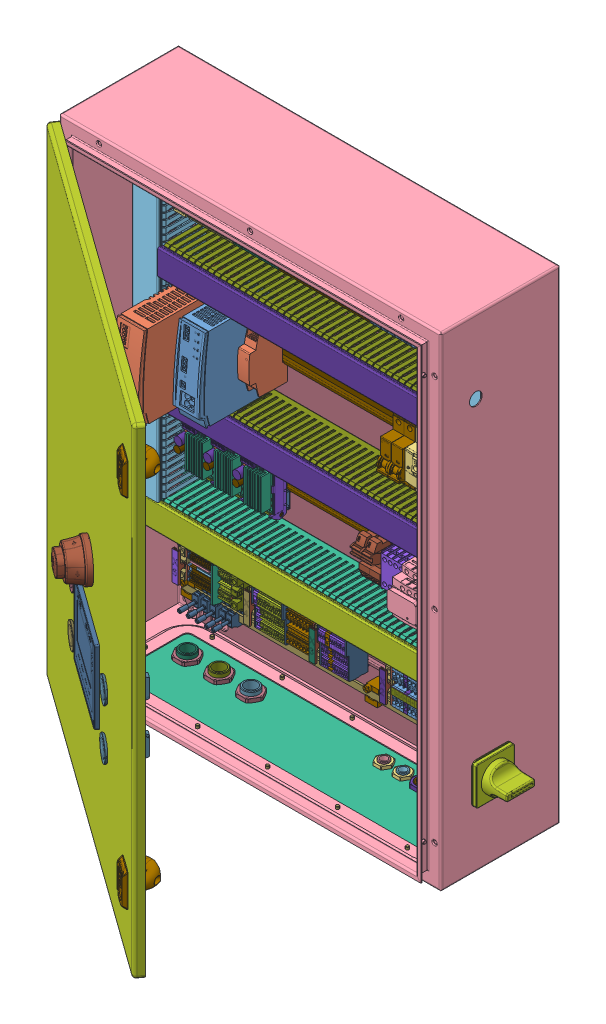
SolidWorks assembly Armoir életrique v46.step, configuration Valor predeterminado. Lengths in mm. (continued)
Components (placement in the parent): (continued)
- 37.5 X 75 Narrow Slot BASE WITH LID.step-1: 37.5 X 75 Narrow Slot BASE WITH LID.step [Valor predeterminado] at origin size (468 41.01 78.6)
  - Body1.step-1: Body1.step [Valor predeterminado] at (-551 554.8681 -521.8) x (0 -1 0) z (0 0 1) size (41 468 77)
  - Body2.step-1: Body2.step [Valor predeterminado] at (-551 554.8681 -521.8) x (0 -1 0) z (0 0 1) size (41.01 468 7.4)
- 37.5 X 75 Narrow Slot BASE WITH LID_1.step-1: 37.5 X 75 Narrow Slot BASE WITH LID_1.step [Valor predeterminado] at (0 -220 0) size (468 41.01 78.6)
  - Body1.step-1: Body1.step [Valor predeterminado] at (-551 593.8681 -521.8) x (0 -1 0) z (0 0 1) size (41 468 77)
  - Body2.step-1: Body2.step [Valor predeterminado] at (-551 593.8681 -521.8) x (0 -1 0) z (0 0 1) size (41.01 468 7.4)
- 1207653 466.step-1: 1207653 466.step [Valor predeterminado] at (0 375 125) size (466 35 7.5)
  - NS_35_7.5_PERF_955MM-select.step-1: NS_35_7.5_PERF_955MM-select.step [Valor predeterminado] at (125.3 207.4662 -151.4677) x (0 1 0) z (1 0 0) size (35 7.5 466)
- 1207653 466_1.step-1: 1207653 466_1.step [Valor predeterminado] at (0 145 125) size (466 35 7.5)
  - NS_35_7.5_PERF_955MM-select.step-1: NS_35_7.5_PERF_955MM-select.step [Valor predeterminado] at (126.3 85.9654 -151.4677) x (0 1 0) z (1 0 0) size (35 7.5 466)
- 2905743.step-1: 2905743.step [Valor predeterminado] at (0 550 200) size (41 130.04 121)
  - CBM_E4_24DC_0.5_10A_NO_R-select.step-1: CBM_E4_24DC_0.5_10A_NO_R-select.step [Valor predeterminado] at (132.998 -56.1004 -52.502) x (0 0 -1) z (0 -1 0) size (121 41 130.04)
- 2903149_TRIO_PS_2G_1AC_24DC_10-select.step-1: 2903149_TRIO_PS_2G_1AC_24DC_10-select.step [Valor predeterminado] at (50 625 200) x (0 1 0) z (1 0 0) size (130 167 42)
  - 2903149_TRIO_PS_2G_1AC_24DC_10-select_1.step-1: 2903149_TRIO_PS_2G_1AC_24DC_10-select_1.step [Valor predeterminado] at (-236.8504 -172.5 20.5) x (0 1 0) z (0 0 -1) size (167 130 42)
- 37.5 X 75 Narrow Slot BASE WITH LID_2.step-1: 37.5 X 75 Narrow Slot BASE WITH LID_2.step [Valor predeterminado] at (0 -500 0) size (468 41.01 78.6)
  - Body1.step-1: Body1.step [Valor predeterminado] at (-550 694.8677 -521.8) x (0 -1 0) z (0 0 1) size (41 468 77)
  - Body2.step-1: Body2.step [Valor predeterminado] at (-550 694.8677 -521.8) x (0 -1 0) z (0 0 1) size (41.01 468 7.4)
- 1207653 466_2.step-1: 1207653 466_2.step [Valor predeterminado] at (0 -145 125) size (466 35 7.5)
  - NS_35_7.5_PERF_955MM-select.step-1: NS_35_7.5_PERF_955MM-select.step [Valor predeterminado] at (125.3 544.9658 -151.4677) x (0 1 0) z (1 0 0) size (35 7.5 466)
- 2903334_RIF_1_RPT_LDP_24DC_2x21-select_1.step-1: 2903334_RIF_1_RPT_LDP_24DC_2x21-select_1.step [Valor predeterminado] at (240 390 50) x (0 1 0) z (1 0 0) size (104.84 89.77 16.3)
  - 2903334_RIF_1_RPT_LDP_24DC_2x21-select_2.step-1: 2903334_RIF_1_RPT_LDP_24DC_2x21-select_2.step [Valor predeterminado] at (-71.3019 -22.3322 159.95) x (-0.992546 -0.121869 0) z (0 0 -1) size (95.96 78.66 16.3)
- GV2ME16.step-1: GV2ME16.step [Valor predeterminado] at origin size (89 89 77.76)
  - GV2ME10-3D-SIMPLIFIED.step-1: GV2ME10-3D-SIMPLIFIED.step [Valor predeterminado] at (463.25 407.4996 47.5) size (44.5 89 77.76)
  - GV2ME10-3D-SIMPLIFIED.step-2: GV2ME10-3D-SIMPLIFIED.step [Valor predeterminado] at (507.75 407.4996 47.5) size (44.5 89 77.76)
- LC1D12BD.step-1: LC1D12BD.step [Valor predeterminado] at (700 300 0) size (89.6 77 94.65)
  - LC1D09-18C-DC.step-1: LC1D09-18C-DC.step [Valor predeterminado] at (-258.6 -55.7008 22) size (44.8 77 94.65)
  - LC1D09-18C-DC.step-2: LC1D09-18C-DC.step [Valor predeterminado] at (-213.8 -55.7008 22) size (44.8 77 94.65)
- 37.5 X 75 Narrow Slot BASE WITH LID_3.step-1: 37.5 X 75 Narrow Slot BASE WITH LID_3.step [Valor predeterminado] at origin size (41.01 529 78.6)
  - Body1_1.step-1: Body1_1.step [Valor predeterminado] at (211.6315 -337.5 -521.8) size (41.01 529 78.6)
- 37.5 X 75 Narrow Slot BASE WITH LID_4.step-1: 37.5 X 75 Narrow Slot BASE WITH LID_4.step [Valor predeterminado] at (350 0 0) size (41.01 529 78.6)
  - Body1_1.step-1: Body1_1.step [Valor predeterminado] at (370.6319 -337.5 -521.8) size (41.01 529 78.6)
- 37.5 X 75 Narrow Slot BASE WITH LID_5.step-1: 37.5 X 75 Narrow Slot BASE WITH LID_5.step [Valor predeterminado] at origin size (550 41.01 78.6)
  - Body1_2.step-1: Body1_2.step [Valor predeterminado] at (-510.0004 25.8681 -521.8) x (0 -1 0) z (0 0 1) size (41 550 77)
  - Body2_2.step-1: Body2_2.step [Valor predeterminado] at (-510.0004 25.8681 -521.8) x (0 -1 0) z (0 0 1) size (41.01 550 7.4)
- Rail bornier complet.step-1: Rail bornier complet.step [Valor predeterminado] at (531.5 121.5 20) x (-1 0 0) z (0 0 1) size (500.55 113.8 62.99)
  - Bornier X3.step-1: Bornier X3.step [Valor predeterminado] at (226.5 -28.5 -20) size (55.9 81.82 53.31)
    - pxc_3244449_03_PTIO-1-5-S-3-PE_3D.step-1: pxc_3244449_03_PTIO-1-5-S-3-PE_3D.step [Valor predeterminado] at origin size (3.5 81.82 53.31)
      - PTIO_1.5_S_3_PE-select.step-1: PTIO_1.5_S_3_PE-select.step [Valor predeterminado] at (9.4 -10.4554 38.8743) x (0 0.992546 -0.121869) z (1 0 0) size (77 44.26 3.5)
    - pxc_3244560_03_PTIO-IN-2-5-3-PE-OG_3D.step-1: pxc_3244560_03_PTIO-IN-2-5-3-PE-OG_3D.step [Valor predeterminado] at (12 0 0) size (7 74.4 40)
      - PTIO_IN_2.5_3_PE_OG-Select.step-1: PTIO_IN_2.5_3_PE_OG-Select.step [Valor predeterminado] at (-50.17 -12.4414 42.0332) x (0 1 0) z (1 0 0) size (74.4 40 7)
    - pxc_3244449_03_PTIO-1-5-S-3-PE_3D_1.step-1: pxc_3244449_03_PTIO-1-5-S-3-PE_3D_1.step [Valor predeterminado] at (-25 0 0) size (3.5 81.82 53.31)
      - PTIO_1.5_S_3_PE-select.step-1: PTIO_1.5_S_3_PE-select.step [Valor predeterminado] at (30.9 -10.4554 38.8743) x (0 0.992546 -0.121869) z (1 0 0) size (77 44.26 3.5)
    - pxc_3244449_03_PTIO-1-5-S-3-PE_3D_2.step-1: pxc_3244449_03_PTIO-1-5-S-3-PE_3D_2.step [Valor predeterminado] at (-45 0 0) size (3.5 81.82 53.31)
      - PTIO_1.5_S_3_PE-select.step-1: PTIO_1.5_S_3_PE-select.step [Valor predeterminado] at (64.9 -10.4554 38.8743) x (0 0.992546 -0.121869) z (1 0 0) size (77 44.26 3.5)
    - pxc_3244449_03_PTIO-1-5-S-3-PE_3D_3.step-1: pxc_3244449_03_PTIO-1-5-S-3-PE_3D_3.step [Valor predeterminado] at (-37 0 0) size (3.5 81.82 53.31)
      - PTIO_1.5_S_3_PE-select.step-1: PTIO_1.5_S_3_PE-select.step [Valor predeterminado] at (60.4 -10.4554 38.8743) x (0 0.992546 -0.121869) z (1 0 0) size (77 44.26 3.5)
    - pxc_3244449_03_PTIO-1-5-S-3-PE_3D_4.step-1: pxc_3244449_03_PTIO-1-5-S-3-PE_3D_4.step [Valor predeterminado] at (-60 0 0) size (3.5 81.82 53.31)
      - PTIO_1.5_S_3_PE-select.step-1: PTIO_1.5_S_3_PE-select.step [Valor predeterminado] at (62.4 -10.4554 38.8743) x (0 0.992546 -0.121869) z (1 0 0) size (77 44.26 3.5)
    - pxc_3244449_03_PTIO-1-5-S-3-PE_3D_5.step-1: pxc_3244449_03_PTIO-1-5-S-3-PE_3D_5.step [Valor predeterminado] at (-76 0 0) size (3.5 81.82 53.31)
      - PTIO_1.5_S_3_PE-select.step-1: PTIO_1.5_S_3_PE-select.step [Valor predeterminado] at (74.9 -10.4554 38.8743) x (0 0.992546 -0.121869) z (1 0 0) size (77 44.26 3.5)
    - pxc_3244449_03_PTIO-1-5-S-3-PE_3D_6.step-1: pxc_3244449_03_PTIO-1-5-S-3-PE_3D_6.step [Valor predeterminado] at (-93 0 0) size (3.5 81.82 53.31)
      - PTIO_1.5_S_3_PE-select.step-1: PTIO_1.5_S_3_PE-select.step [Valor predeterminado] at (88.4 -10.4554 38.8743) x (0 0.992546 -0.121869) z (1 0 0) size (77 44.26 3.5)
    - pxc_3244449_03_PTIO-1-5-S-3-PE_3D_7.step-1: pxc_3244449_03_PTIO-1-5-S-3-PE_3D_7.step [Valor predeterminado] at (-107 0 0) size (3.5 81.82 53.31)
      - PTIO_1.5_S_3_PE-select.step-1: PTIO_1.5_S_3_PE-select.step [Valor predeterminado] at (98.9 -10.4554 38.8743) x (0 0.992546 -0.121869) z (1 0 0) size (77 44.26 3.5)
    - pxc_3244449_03_PTIO-1-5-S-3-PE_3D_8.step-1: pxc_3244449_03_PTIO-1-5-S-3-PE_3D_8.step [Valor predeterminado] at (-121 0 0) size (3.5 81.82 53.31)
      - PTIO_1.5_S_3_PE-select.step-1: PTIO_1.5_S_3_PE-select.step [Valor predeterminado] at (109.4 -10.4554 38.8743) x (0 0.992546 -0.121869) z (1 0 0) size (77 44.26 3.5)
    - pxc_3244575_01_D-PTIO-1-5-S-3_3D.step-1: pxc_3244575_01_D-PTIO-1-5-S-3_3D.step [Valor predeterminado] at (5 -8 5) size (2.2 74.4 33.8)
      - D_PTIO_1.5_S_3-select.step-1: D_PTIO_1.5_S_3-select.step [Valor predeterminado] at (-28.27 26.0888 49.1305) x (0 1 0) z (1 0 0) size (74.4 33.8 2.2)
    - pxc_3244575_01_D-PTIO-1-5-S-3_3D_1.step-1: pxc_3244575_01_D-PTIO-1-5-S-3_3D_1.step [Valor predeterminado] at (-60 -8 5) size (2.2 74.4 33.8)
      - D_PTIO_1.5_S_3-select.step-1: D_PTIO_1.5_S_3-select.step [Valor predeterminado] at (-7.47 26.0888 49.1305) x (0 1 0) z (1 0 0) size (74.4 33.8 2.2)
    - pxc_1202577_02_E-UK-NS-35_3D.step-1: pxc_1202577_02_E-UK-NS-35_3D.step [Valor predeterminado] at (8 0 0) size (9.5 54 43.4)
      - pxc_1004348_03_KLM-A_3D.step-1: pxc_1004348_03_KLM-A_3D.step [Valor predeterminado] at (0 0 7) size (9.5 46 36.8)
        - KLM_A-select.step-1: KLM_A-select.step [Valor predeterminado] at (21.1 -2.3378 32.5) x (0 1 0) z (1 0 0) size (46 36.8 9.5)
      - E_UK_NS_35_select.step-1: E_UK_NS_35_select.step [Valor predeterminado] at (21.1 448.4984 -308.7806) x (0 1 0) z (1 0 0) size (54 34.6 9.5)
    - pxc_3244449_03_PTIO-1-5-S-3-PE_3D_9.step-1: pxc_3244449_03_PTIO-1-5-S-3-PE_3D_9.step [Valor predeterminado] at (-26 0 0) size (3.5 81.82 53.31)
      - PTIO_1.5_S_3_PE-select.step-1: PTIO_1.5_S_3_PE-select.step [Valor predeterminado] at (52.9 -10.4554 38.8743) x (0 0.992546 -0.121869) z (1 0 0) size (77 44.26 3.5)
    - pxc_3213125_03_FBS-10-3-5-BU_3D.step-1: pxc_3213125_03_FBS-10-3-5-BU_3D.step [Valor predeterminado] at (0 0 60) size (26.75 3 18.23)
      - FBS_10_3.5_BU-select.step-1: FBS_10_3.5_BU-select.step [Valor predeterminado] at (38.285 40.9822 6.575) x (0 -1 0) z (-1 0 0) size (3 18.22 26.75)
    - pxc_3213109_03_FBS-4-3-5-BU_3D.step-1: pxc_3213109_03_FBS-4-3-5-BU_3D.step [Valor predeterminado] at (0 0 40) size (12.75 3 18.23)
      - FBS_4_3.5_BU-select.step-1: FBS_4_3.5_BU-select.step [Valor predeterminado] at (-33.485 32.7678 26.575) x (0 1 0) z (1 0 0) size (3 18.22 12.75)
    - Etiquette X3.step-1: Etiquette X3.step [Valor predeterminado] at (38.6 65 64.5) x (-1 0 0) z (0 0 1) size (9.5 46 0.1)
  - Bornier Alim.step-1: Bornier Alim.step [Valor predeterminado] at (81.5 -28.5 -20) size (54.15 55.92 43.5)
    - pxc_1202577_02_E-UK-NS-35_3D_1.step-1: pxc_1202577_02_E-UK-NS-35_3D_1.step [Valor predeterminado] at (0 0 -44) size (9.5 54 43.4)
      - pxc_1004348_03_KLM-A_3D_1.step-1: pxc_1004348_03_KLM-A_3D_1.step [Valor predeterminado] at (0 0 7) size (9.5 46 36.8)
        - KLM_A-select.step-1: KLM_A-select.step [Valor predeterminado] at (-36.85 -2.3378 76.5) x (0 1 0) z (1 0 0) size (46 36.8 9.5)
      - E_UK_NS_35_select.step-1: E_UK_NS_35_select.step [Valor predeterminado] at (-36.85 448.4984 -264.7806) x (0 1 0) z (1 0 0) size (54 34.6 9.5)
    - pxc_1202577_02_E-UK-NS-35_3D_2.step-1: pxc_1202577_02_E-UK-NS-35_3D_2.step [Valor predeterminado] at (0 0 52) size (9.5 54 34.6)
      - E_UK_NS_35_select_1.step-1: E_UK_NS_35_select_1.step [Valor predeterminado] at (-81.5 448.4984 -360.7806) x (0 1 0) z (1 0 0) size (54 34.6 9.5)
    - pxc_3211766_13_PT-4-PE_3D.step-1: pxc_3211766_13_PT-4-PE_3D.step [Valor predeterminado] at origin size (6.15 55.9 35.25)
      - PT_4_PE-select.step-1: PT_4_PE-select.step [Valor predeterminado] at (-64.65 61.3 36.75) x (0 1 0) z (1 0 0) size (55.9 35.25 6.15)
    - pxc_3211760_14_PT-4-BU_3D.step-1: pxc_3211760_14_PT-4-BU_3D.step [Valor predeterminado] at (-12 0 0) size (6.15 55.9 35.25)
      - PT_4_BU-Select.step-1: PT_4_BU-Select.step [Valor predeterminado] at (-46.5 61.3 36.75) x (0 1 0) z (1 0 0) size (55.9 35.25 6.15)
    - pxc_3211757_14_PT-4_3D.step-1: pxc_3211757_14_PT-4_3D.step [Valor predeterminado] at (-30 0 0) size (6.15 55.9 35.25)
      - PT_4-Select.step-1: PT_4-Select.step [Valor predeterminado] at (-10.05 61.3 36.75) x (0 1 0) z (1 0 0) size (55.9 35.25 6.15)
    - pxc_3211757_14_PT-4_3D_1.step-1: pxc_3211757_14_PT-4_3D_1.step [Valor predeterminado] at (-43 0 0) size (6.15 55.9 35.25)
      - PT_4-Select.step-1: PT_4-Select.step [Valor predeterminado] at (-3.2 61.3 36.75) x (0 1 0) z (1 0 0) size (55.9 35.25 6.15)
    - pxc_3211757_14_PT-4_3D_2.step-1: pxc_3211757_14_PT-4_3D_2.step [Valor predeterminado] at (-54 0 0) size (6.15 55.9 35.25)
      - PT_4-Select.step-1: PT_4-Select.step [Valor predeterminado] at (1.65 61.3 36.75) x (0 1 0) z (1 0 0) size (55.9 35.25 6.15)
    - pxc_3030420_04_D-ST-4_3D.step-1: pxc_3030420_04_D-ST-4_3D.step [Valor predeterminado] at (-40 0 0) size (2.2 55.9 29.05)
      - D-ST4-Body.step-1: D-ST4-Body.step [Valor predeterminado] at (-32 2.4502 65.8799) x (0 1 0) z (1 0 0) size (55.9 29.05 2.2)
      - D-ST4_Bridge_element1.step-1: D-ST4_Bridge_element1.step [Valor predeterminado] at (-32 2.4502 65.8799) x (0 1 0) z (1 0 0) size (9.39 5.98 1.8)
    - pxc_3030420_04_D-ST-4_3D_1.step-1: pxc_3030420_04_D-ST-4_3D_1.step [Valor predeterminado] at (-40 0 0) size (2.2 55.9 29.05)
      - D-ST4-Body.step-1: D-ST4-Body.step [Valor predeterminado] at (0.95 2.4502 65.8799) x (0 1 0) z (1 0 0) size (55.9 29.05 2.2)
      - D-ST4_Bridge_element1.step-1: D-ST4_Bridge_element1.step [Valor predeterminado] at (0.95 2.4502 65.8799) x (0 1 0) z (1 0 0) size (9.39 5.98 1.8)
    - Reperage X1.step-1: Reperage X1.step [Valor predeterminado] at (-61 45 40) x (0 -1 0) z (-1 0 0) size (10.5 4.25 30.75)
      - pxc_1051414_01_ZB-6-LGS-L1-N-PE_3D.step-1: pxc_1051414_01_ZB-6-LGS-L1-N-PE_3D.step [Valor predeterminado] at origin size (10.5 4.2 6.15)
        - 1051003_ZB_6_UNBEDRUCKT-select.step-1: 1051003_ZB_6_UNBEDRUCKT-select.step [Valor predeterminado] at (1061.9663 -328.6937 -21.95) size (10.5 4.2 6.15)
      - pxc_1051414_01_ZB-6-LGS-L1-N-PE_3D_1.step-1: pxc_1051414_01_ZB-6-LGS-L1-N-PE_3D_1.step [Valor predeterminado] at (8 0 0) size (10.5 4.2 6.15)
        - 1051003_ZB_6_UNBEDRUCKT-select.step-1: 1051003_ZB_6_UNBEDRUCKT-select.step [Valor predeterminado] at (1053.9663 -328.6937 -15.8) size (10.5 4.2 6.15)
      - pxc_1051414_01_ZB-6-LGS-L1-N-PE_3D_2.step-1: pxc_1051414_01_ZB-6-LGS-L1-N-PE_3D_2.step [Valor predeterminado] at (16 0 0) size (10.5 4.2 6.15)
        - 1051003_ZB_6_UNBEDRUCKT-select.step-1: 1051003_ZB_6_UNBEDRUCKT-select.step [Valor predeterminado] at (1045.9663 -328.6937 -9.65) size (10.5 4.2 6.15)
      - pxc_1051414_01_ZB-6-LGS-L1-N-PE_3D_3.step-1: pxc_1051414_01_ZB-6-LGS-L1-N-PE_3D_3.step [Valor predeterminado] at (24 0 0) size (10.5 4.2 6.15)
        - 1051003_ZB_6_UNBEDRUCKT-select.step-1: 1051003_ZB_6_UNBEDRUCKT-select.step [Valor predeterminado] at (1037.9663 -328.6937 -3.5) size (10.5 4.2 6.15)
      - pxc_1051414_01_ZB-6-LGS-L1-N-PE_3D_4.step-1: pxc_1051414_01_ZB-6-LGS-L1-N-PE_3D_4.step [Valor predeterminado] at (33 0 0) size (10.5 4.2 6.15)
        - 1051003_ZB_6_UNBEDRUCKT-select.step-1: 1051003_ZB_6_UNBEDRUCKT-select.step [Valor predeterminado] at (1028.9663 -328.6937 2.65) size (10.5 4.2 6.15)
      - Etiquette X1 1.step-1: Etiquette X1 1.step [Valor predeterminado] at (-7.5185 17.85 -21.95) x (0 0 1) z (0 1 0) size (30.75 10.5 0.05)
    - Etiquette X1.step-1: Etiquette X1.step [Valor predeterminado] at (-27.35 65 64.5) x (-1 0 0) z (0 0 1) size (9.5 46 0.1)
  - Bornier X4.step-1: Bornier X4.step [Valor predeterminado] at (266.5 -28.5 -20) size (102.8 81.82 53.31)
    - pxc_1202577_02_E-UK-NS-35_3D_3.step-1: pxc_1202577_02_E-UK-NS-35_3D_3.step [Valor predeterminado] at (90 0 0) size (9.5 54 43.4)
      - pxc_1004348_03_KLM-A_3D_2.step-1: pxc_1004348_03_KLM-A_3D_2.step [Valor predeterminado] at (0 0 7) size (9.5 46 36.8)
        - KLM_A-select.step-1: KLM_A-select.step [Valor predeterminado] at (1.9 -2.3378 32.5) x (0 1 0) z (1 0 0) size (46 36.8 9.5)
      - E_UK_NS_35_select.step-1: E_UK_NS_35_select.step [Valor predeterminado] at (1.9 448.4984 -308.7806) x (0 1 0) z (1 0 0) size (54 34.6 9.5)
    - pxc_3244436_03_PTIO-1-5-S-3-LED-24-GN_3D.step-1: pxc_3244436_03_PTIO-1-5-S-3-LED-24-GN_3D.step [Valor predeterminado] at (60 0 55) size (3.5 81.82 53.31)
      - PTIO_1.5_S_3_LED_24_GN-select.step-1: PTIO_1.5_S_3_LED_24_GN-select.step [Valor predeterminado] at (22.7 -10.4554 -16.1257) x (0 0.992546 -0.121869) z (1 0 0) size (77 44.26 3.5)
    - pxc_3244436_03_PTIO-1-5-S-3-LED-24-GN_3D_1.step-1: pxc_3244436_03_PTIO-1-5-S-3-LED-24-GN_3D_1.step [Valor predeterminado] at (55 0 55) size (3.5 81.82 53.31)
      - PTIO_1.5_S_3_LED_24_GN-select.step-1: PTIO_1.5_S_3_LED_24_GN-select.step [Valor predeterminado] at (24.2 -10.4554 -16.1257) x (0 0.992546 -0.121869) z (1 0 0) size (77 44.26 3.5)
    - pxc_3244436_03_PTIO-1-5-S-3-LED-24-GN_3D_2.step-1: pxc_3244436_03_PTIO-1-5-S-3-LED-24-GN_3D_2.step [Valor predeterminado] at (50 0 55) size (3.5 81.82 53.31)
      - PTIO_1.5_S_3_LED_24_GN-select.step-1: PTIO_1.5_S_3_LED_24_GN-select.step [Valor predeterminado] at (25.7 -10.4554 -16.1257) x (0 0.992546 -0.121869) z (1 0 0) size (77 44.26 3.5)
    - pxc_3244436_03_PTIO-1-5-S-3-LED-24-GN_3D_3.step-1: pxc_3244436_03_PTIO-1-5-S-3-LED-24-GN_3D_3.step [Valor predeterminado] at (45 0 55) size (3.5 81.82 53.31)
      - PTIO_1.5_S_3_LED_24_GN-select.step-1: PTIO_1.5_S_3_LED_24_GN-select.step [Valor predeterminado] at (27.2 -10.4554 -16.1257) x (0 0.992546 -0.121869) z (1 0 0) size (77 44.26 3.5)
    - pxc_3244559_05_PTIO-IN-2-5-3-OG_3D.step-1: pxc_3244559_05_PTIO-IN-2-5-3-OG_3D.step [Valor predeterminado] at (85 0 55) size (7 74.4 40)
      - PTIO_IN_2.5_3_OG-select.step-1: PTIO_IN_2.5_3_OG-select.step [Valor predeterminado] at (-49.87 -12.4414 -12.9668) x (0 1 0) z (1 0 0) size (74.4 40 7)
    - pxc_3244436_03_PTIO-1-5-S-3-LED-24-GN_3D_4.step-1: pxc_3244436_03_PTIO-1-5-S-3-LED-24-GN_3D_4.step [Valor predeterminado] at (45 0 55) size (3.5 81.82 53.31)
      - PTIO_1.5_S_3_LED_24_GN-select.step-1: PTIO_1.5_S_3_LED_24_GN-select.step [Valor predeterminado] at (23.7 -10.4554 -16.1257) x (0 0.992546 -0.121869) z (1 0 0) size (77 44.26 3.5)
    - pxc_3244436_03_PTIO-1-5-S-3-LED-24-GN_3D_5.step-1: pxc_3244436_03_PTIO-1-5-S-3-LED-24-GN_3D_5.step [Valor predeterminado] at (35 0 55) size (3.5 81.82 53.31)
      - PTIO_1.5_S_3_LED_24_GN-select.step-1: PTIO_1.5_S_3_LED_24_GN-select.step [Valor predeterminado] at (30.2 -10.4554 -16.1257) x (0 0.992546 -0.121869) z (1 0 0) size (77 44.26 3.5)
    - pxc_3244436_03_PTIO-1-5-S-3-LED-24-GN_3D_6.step-1: pxc_3244436_03_PTIO-1-5-S-3-LED-24-GN_3D_6.step [Valor predeterminado] at (25 0 55) size (3.5 81.82 53.31)
      - PTIO_1.5_S_3_LED_24_GN-select.step-1: PTIO_1.5_S_3_LED_24_GN-select.step [Valor predeterminado] at (36.7 -10.4554 -16.1257) x (0 0.992546 -0.121869) z (1 0 0) size (77 44.26 3.5)
    - pxc_3244436_03_PTIO-1-5-S-3-LED-24-GN_3D_7.step-1: pxc_3244436_03_PTIO-1-5-S-3-LED-24-GN_3D_7.step [Valor predeterminado] at (20 0 55) size (3.5 81.82 53.31)
      - PTIO_1.5_S_3_LED_24_GN-select.step-1: PTIO_1.5_S_3_LED_24_GN-select.step [Valor predeterminado] at (38.2 -10.4554 -16.1257) x (0 0.992546 -0.121869) z (1 0 0) size (77 44.26 3.5)
    - pxc_3244436_03_PTIO-1-5-S-3-LED-24-GN_3D_8.step-1: pxc_3244436_03_PTIO-1-5-S-3-LED-24-GN_3D_8.step [Valor predeterminado] at (15 0 55) size (3.5 81.82 53.31)
      - PTIO_1.5_S_3_LED_24_GN-select.step-1: PTIO_1.5_S_3_LED_24_GN-select.step [Valor predeterminado] at (39.7 -10.4554 -16.1257) x (0 0.992546 -0.121869) z (1 0 0) size (77 44.26 3.5)
    - pxc_3244436_03_PTIO-1-5-S-3-LED-24-GN_3D_9.step-1: pxc_3244436_03_PTIO-1-5-S-3-LED-24-GN_3D_9.step [Valor predeterminado] at (10 0 55) size (3.5 81.82 53.31)
      - PTIO_1.5_S_3_LED_24_GN-select.step-1: PTIO_1.5_S_3_LED_24_GN-select.step [Valor predeterminado] at (41.2 -10.4554 -16.1257) x (0 0.992546 -0.121869) z (1 0 0) size (77 44.26 3.5)
    - pxc_3244436_03_PTIO-1-5-S-3-LED-24-GN_3D_10.step-1: pxc_3244436_03_PTIO-1-5-S-3-LED-24-GN_3D_10.step [Valor predeterminado] at (35 0 55) size (3.5 81.82 53.31)
      - PTIO_1.5_S_3_LED_24_GN-select.step-1: PTIO_1.5_S_3_LED_24_GN-select.step [Valor predeterminado] at (12.7 -10.4554 -16.1257) x (0 0.992546 -0.121869) z (1 0 0) size (77 44.26 3.5)
    - pxc_3244575_01_D-PTIO-1-5-S-3_3D_2.step-1: pxc_3244575_01_D-PTIO-1-5-S-3_3D_2.step [Valor predeterminado] at origin size (2.2 74.4 33.8)
      - D_PTIO_1.5_S_3-select.step-1: D_PTIO_1.5_S_3-select.step [Valor predeterminado] at (39.53 18.0888 54.1305) x (0 1 0) z (1 0 0) size (74.4 33.8 2.2)
    - pxc_3244575_01_D-PTIO-1-5-S-3_3D_3.step-1: pxc_3244575_01_D-PTIO-1-5-S-3_3D_3.step [Valor predeterminado] at (25 0 0) size (2.2 74.4 33.8)
      - D_PTIO_1.5_S_3-select.step-1: D_PTIO_1.5_S_3-select.step [Valor predeterminado] at (-33.17 18.0888 54.1305) x (0 1 0) z (1 0 0) size (74.4 33.8 2.2)
    - pxc_3212329_18_PT-2-5-OG_3D.step-1: pxc_3212329_18_PT-2-5-OG_3D.step [Valor predeterminado] at (75 0 0) size (5.15 55.36 46.64)
      - PT_2.5_OG-select.step-1: PT_2.5_OG-select.step [Valor predeterminado] at (-33 7.1011 27.6678) x (0 0.992546 -0.121869) z (1 0 0) size (50.77 40.76 5.15)
    - pxc_3212329_18_PT-2-5-OG_3D_1.step-1: pxc_3212329_18_PT-2-5-OG_3D_1.step [Valor predeterminado] at (60 0 0) size (5.15 55.36 46.64)
      - PT_2.5_OG-select.step-1: PT_2.5_OG-select.step [Valor predeterminado] at (-23.15 7.1011 27.6678) x (0 0.992546 -0.121869) z (1 0 0) size (50.77 40.76 5.15)
    - pxc_3212329_18_PT-2-5-OG_3D_2.step-1: pxc_3212329_18_PT-2-5-OG_3D_2.step [Valor predeterminado] at (47 0 0) size (5.15 55.36 46.64)
      - PT_2.5_OG-select.step-1: PT_2.5_OG-select.step [Valor predeterminado] at (-15.3 7.1011 27.6678) x (0 0.992546 -0.121869) z (1 0 0) size (50.77 40.76 5.15)
    - pxc_3212329_18_PT-2-5-OG_3D_3.step-1: pxc_3212329_18_PT-2-5-OG_3D_3.step [Valor predeterminado] at (36 0 0) size (5.15 55.36 46.64)
      - PT_2.5_OG-select.step-1: PT_2.5_OG-select.step [Valor predeterminado] at (-9.45 7.1011 27.6678) x (0 0.992546 -0.121869) z (1 0 0) size (50.77 40.76 5.15)
    - pxc_3212329_18_PT-2-5-OG_3D_4.step-1: pxc_3212329_18_PT-2-5-OG_3D_4.step [Valor predeterminado] at (26 0 0) size (5.15 55.36 46.64)
      - PT_2.5_OG-select.step-1: PT_2.5_OG-select.step [Valor predeterminado] at (-4.6 7.1011 27.6678) x (0 0.992546 -0.121869) z (1 0 0) size (50.77 40.76 5.15)
    - pxc_3212329_18_PT-2-5-OG_3D_5.step-1: pxc_3212329_18_PT-2-5-OG_3D_5.step [Valor predeterminado] at (14 0 0) size (5.15 55.36 46.64)
      - PT_2.5_OG-select.step-1: PT_2.5_OG-select.step [Valor predeterminado] at (2.25 7.1011 27.6678) x (0 0.992546 -0.121869) z (1 0 0) size (50.77 40.76 5.15)
    - pxc_3212329_18_PT-2-5-OG_3D_6.step-1: pxc_3212329_18_PT-2-5-OG_3D_6.step [Valor predeterminado] at (14 0 0) size (5.15 55.36 46.64)
      - PT_2.5_OG-select.step-1: PT_2.5_OG-select.step [Valor predeterminado] at (-2.9 7.1011 27.6678) x (0 0.992546 -0.121869) z (1 0 0) size (50.77 40.76 5.15)
    - pxc_3212329_18_PT-2-5-OG_3D_7.step-1: pxc_3212329_18_PT-2-5-OG_3D_7.step [Valor predeterminado] at (4 0 0) size (5.15 55.36 46.64)
      - PT_2.5_OG-select.step-1: PT_2.5_OG-select.step [Valor predeterminado] at (1.95 7.1011 27.6678) x (0 0.992546 -0.121869) z (1 0 0) size (50.77 40.76 5.15)
    - pxc_3030417_05_D-ST-2-5_3D.step-1: pxc_3030417_05_D-ST-2-5_3D.step [Valor predeterminado] at (-5 0 0) size (2.2 48.6 29.05)
      - D-ST_2.5-Bridge_element1.step-1: D-ST_2.5-Bridge_element1.step [Valor predeterminado] at (3.6 6.3703 65.9) x (0 1 0) z (1 0 0) size (9.44 6 1.8)
      - D-ST_2.5-Body.step-1: D-ST_2.5-Body.step [Valor predeterminado] at (3.6 6.3703 65.9) x (0 1 0) z (1 0 0) size (48.6 29.05 2.2)
    - Etiquette X4.step-1: Etiquette X4.step [Valor predeterminado] at (101.4 65 64.5) x (-1 0 0) z (0 0 1) size (9.5 46 0.1)
  - 1207653.step-1: 1207653.step [Valor predeterminado] at (81.5 -28.5 -20) size (480 35 7.5)
    - NS_35_7.5_PERF_955MM-select_1.step-1: NS_35_7.5_PERF_955MM-select_1.step [Valor predeterminado] at (-20.2 -9.0338 -26.4677) x (0 1 0) z (1 0 0) size (35 7.5 480)
  - Bornier X2 moteur.step-1: Bornier X2 moteur.step [Valor predeterminado] at (112.5 -28.5 -20) size (100 55.92 43.5)
    - pxc_1202577_02_E-UK-NS-35_3D_4.step-1: pxc_1202577_02_E-UK-NS-35_3D_4.step [Valor predeterminado] at (0 0 -109) size (9.5 54 43.4)
      - pxc_1004348_03_KLM-A_3D_3.step-1: pxc_1004348_03_KLM-A_3D_3.step [Valor predeterminado] at (0 0 7) size (9.5 46 36.8)
        - KLM_A-select.step-1: KLM_A-select.step [Valor predeterminado] at (32.15 -2.3378 141.5) x (0 1 0) z (1 0 0) size (46 36.8 9.5)
      - E_UK_NS_35_select.step-1: E_UK_NS_35_select.step [Valor predeterminado] at (32.15 448.4984 -199.7806) x (0 1 0) z (1 0 0) size (54 34.6 9.5)
    - pxc_3211757_14_PT-4_3D_3.step-1: pxc_3211757_14_PT-4_3D_3.step [Valor predeterminado] at origin size (6.15 55.9 35.25)
      - PT_4-Select.step-1: PT_4-Select.step [Valor predeterminado] at (-26.4 61.3 36.75) x (0 1 0) z (1 0 0) size (55.9 35.25 6.15)
    - pxc_3211760_14_PT-4-BU_3D_1.step-1: pxc_3211760_14_PT-4-BU_3D_1.step [Valor predeterminado] at (-15 0 0) size (6.15 55.9 35.25)
      - PT_4_BU-Select.step-1: PT_4_BU-Select.step [Valor predeterminado] at (-5.25 61.3 36.75) x (0 1 0) z (1 0 0) size (55.9 35.25 6.15)
    - pxc_3211766_13_PT-4-PE_3D_1.step-1: pxc_3211766_13_PT-4-PE_3D_1.step [Valor predeterminado] at (19 0 0) size (6.15 55.9 35.25)
      - PT_4_PE-select.step-1: PT_4_PE-select.step [Valor predeterminado] at (-33.1 61.3 36.75) x (0 1 0) z (1 0 0) size (55.9 35.25 6.15)
    - pxc_3211766_13_PT-4-PE_3D_2.step-1: pxc_3211766_13_PT-4-PE_3D_2.step [Valor predeterminado] at (-51 0 70) size (6.15 55.9 35.25)
      - PT_4_PE-select.step-1: PT_4_PE-select.step [Valor predeterminado] at (0 61.3 -33.25) x (0 1 0) z (1 0 0) size (55.9 35.25 6.15)
    - pxc_3211766_13_PT-4-PE_3D_3.step-1: pxc_3211766_13_PT-4-PE_3D_3.step [Valor predeterminado] at (19 0 75) size (6.15 55.9 35.25)
      - PT_4_PE-select.step-1: PT_4_PE-select.step [Valor predeterminado] at (-8.5 61.3 -38.25) x (0 1 0) z (1 0 0) size (55.9 35.25 6.15)
    - pxc_3211757_14_PT-4_3D_4.step-1: pxc_3211757_14_PT-4_3D_4.step [Valor predeterminado] at origin size (6.15 55.9 35.25)
      - PT_4-Select.step-1: PT_4-Select.step [Valor predeterminado] at (-1.8 61.3 36.75) x (0 1 0) z (1 0 0) size (55.9 35.25 6.15)
    - pxc_3211757_14_PT-4_3D_5.step-1: pxc_3211757_14_PT-4_3D_5.step [Valor predeterminado] at origin size (6.15 55.9 35.25)
      - PT_4-Select.step-1: PT_4-Select.step [Valor predeterminado] at (16.65 61.3 36.75) x (0 1 0) z (1 0 0) size (55.9 35.25 6.15)
    - pxc_3211757_14_PT-4_3D_6.step-1: pxc_3211757_14_PT-4_3D_6.step [Valor predeterminado] at origin size (6.15 55.9 35.25)
      - PT_4-Select.step-1: PT_4-Select.step [Valor predeterminado] at (28.95 61.3 36.75) x (0 1 0) z (1 0 0) size (55.9 35.25 6.15)
    - pxc_3211757_14_PT-4_3D_7.step-1: pxc_3211757_14_PT-4_3D_7.step [Valor predeterminado] at origin size (6.15 55.9 35.25)
      - PT_4-Select.step-1: PT_4-Select.step [Valor predeterminado] at (4.35 61.3 36.75) x (0 1 0) z (1 0 0) size (55.9 35.25 6.15)
    - pxc_3211757_14_PT-4_3D_8.step-1: pxc_3211757_14_PT-4_3D_8.step [Valor predeterminado] at origin size (6.15 55.9 35.25)
      - PT_4-Select.step-1: PT_4-Select.step [Valor predeterminado] at (22.8 61.3 36.75) x (0 1 0) z (1 0 0) size (55.9 35.25 6.15)
    - pxc_3211757_14_PT-4_3D_9.step-1: pxc_3211757_14_PT-4_3D_9.step [Valor predeterminado] at origin size (6.15 55.9 35.25)
      - PT_4-Select.step-1: PT_4-Select.step [Valor predeterminado] at (-7.95 61.3 36.75) x (0 1 0) z (1 0 0) size (55.9 35.25 6.15)
    - pxc_3030420_04_D-ST-4_3D_2.step-1: pxc_3030420_04_D-ST-4_3D_2.step [Valor predeterminado] at (0 0 60) size (2.2 55.9 29.05)
      - D-ST4-Body.step-1: D-ST4-Body.step [Valor predeterminado] at (29.95 2.4502 5.8799) x (0 1 0) z (1 0 0) size (55.9 29.05 2.2)
      - D-ST4_Bridge_element1.step-1: D-ST4_Bridge_element1.step [Valor predeterminado] at (29.95 2.4502 5.8799) x (0 1 0) z (1 0 0) size (9.39 5.98 1.8)
    - pxc_3030420_04_D-ST-4_3D_3.step-1: pxc_3030420_04_D-ST-4_3D_3.step [Valor predeterminado] at (-110 0 60) size (2.2 55.9 29.05)
      - D-ST4-Body.step-1: D-ST4-Body.step [Valor predeterminado] at (51.65 2.4502 5.8799) x (0 1 0) z (1 0 0) size (55.9 29.05 2.2)
      - D-ST4_Bridge_element1.step-1: D-ST4_Bridge_element1.step [Valor predeterminado] at (51.65 2.4502 5.8799) x (0 1 0) z (1 0 0) size (9.39 5.98 1.8)
    - pxc_3211757_14_PT-4_3D_10.step-1: pxc_3211757_14_PT-4_3D_10.step [Valor predeterminado] at (85 0 0) size (6.15 55.9 35.25)
      - PT_4-Select.step-1: PT_4-Select.step [Valor predeterminado] at (-129.85 61.3 36.75) x (0 1 0) z (1 0 0) size (55.9 35.25 6.15)
    - pxc_3211760_14_PT-4-BU_3D_2.step-1: pxc_3211760_14_PT-4-BU_3D_2.step [Valor predeterminado] at (70 0 0) size (6.15 55.9 35.25)
      - PT_4_BU-Select.step-1: PT_4_BU-Select.step [Valor predeterminado] at (-108.7 61.3 36.75) x (0 1 0) z (1 0 0) size (55.9 35.25 6.15)
    - pxc_3211766_13_PT-4-PE_3D_4.step-1: pxc_3211766_13_PT-4-PE_3D_4.step [Valor predeterminado] at (104 0 0) size (6.15 55.9 35.25)
      - PT_4_PE-select.step-1: PT_4_PE-select.step [Valor predeterminado] at (-136.55 61.3 36.75) x (0 1 0) z (1 0 0) size (55.9 35.25 6.15)
    - pxc_3036958_04_FBS-4-6-BU_3D.step-1: pxc_3036958_04_FBS-4-6-BU_3D.step [Valor predeterminado] at (0 0 65) size (23.1 3 22.98)
      - FBS_4_6_BU-select.step-1: FBS_4_6_BU-select.step [Valor predeterminado] at (17.36 43.9967 1.225) x (0 -1 0) z (-1 0 0) size (3 22.97 23.1)
    - pxc_3030255_06_FBS-4-6_3D.step-1: pxc_3030255_06_FBS-4-6_3D.step [Valor predeterminado] at origin size (23.1 3 22.98)
      - FBS_4-6_select.step-1: FBS_4-6_select.step [Valor predeterminado] at (11.21 38.9822 66.225) x (0 -1 0) z (-1 0 0) size (3 22.98 23.1)
    - Reperage X2.step-1: Reperage X2.step [Valor predeterminado] at (0 0 72) size (86.1 10.5 4.25)
      - pxc_1051414_01_ZB-6-LGS-L1-N-PE_3D_5.step-1: pxc_1051414_01_ZB-6-LGS-L1-N-PE_3D_5.step [Valor predeterminado] at (29.95 52.5185 -18.35) x (-1 0 0) z (0 0 1) size (6.15 10.5 4.2)
        - 1051003_ZB_6_UNBEDRUCKT-select.step-1: 1051003_ZB_6_UNBEDRUCKT-select.step [Valor predeterminado] at (0 1069.4848 -342.3437) x (0 1 0) z (1 0 0) size (10.5 4.2 6.15)
      - pxc_1051414_01_ZB-6-LGS-L1-N-PE_3D_6.step-1: pxc_1051414_01_ZB-6-LGS-L1-N-PE_3D_6.step [Valor predeterminado] at (23.8 52.5185 -18.35) x (-1 0 0) z (0 0 1) size (6.15 10.5 4.2)
        - 1051003_ZB_6_UNBEDRUCKT-select.step-1: 1051003_ZB_6_UNBEDRUCKT-select.step [Valor predeterminado] at (0 1069.4848 -342.3437) x (0 1 0) z (1 0 0) size (10.5 4.2 6.15)
      - pxc_1051414_01_ZB-6-LGS-L1-N-PE_3D_7.step-1: pxc_1051414_01_ZB-6-LGS-L1-N-PE_3D_7.step [Valor predeterminado] at (17.65 52.5185 -18.35) x (-1 0 0) z (0 0 1) size (6.15 10.5 4.2)
        - 1051003_ZB_6_UNBEDRUCKT-select.step-1: 1051003_ZB_6_UNBEDRUCKT-select.step [Valor predeterminado] at (0 1069.4848 -342.3437) x (0 1 0) z (1 0 0) size (10.5 4.2 6.15)
      - pxc_1051414_01_ZB-6-LGS-L1-N-PE_3D_8.step-1: pxc_1051414_01_ZB-6-LGS-L1-N-PE_3D_8.step [Valor predeterminado] at (11.5 52.5185 -18.35) x (-1 0 0) z (0 0 1) size (6.15 10.5 4.2)
        - 1051003_ZB_6_UNBEDRUCKT-select.step-1: 1051003_ZB_6_UNBEDRUCKT-select.step [Valor predeterminado] at (0 1069.4848 -342.3437) x (0 1 0) z (1 0 0) size (10.5 4.2 6.15)
      - pxc_1051414_01_ZB-6-LGS-L1-N-PE_3D_9.step-1: pxc_1051414_01_ZB-6-LGS-L1-N-PE_3D_9.step [Valor predeterminado] at (5.35 52.5185 -18.35) x (-1 0 0) z (0 0 1) size (6.15 10.5 4.2)
        - 1051003_ZB_6_UNBEDRUCKT-select.step-1: 1051003_ZB_6_UNBEDRUCKT-select.step [Valor predeterminado] at (0 1069.4848 -342.3437) x (0 1 0) z (1 0 0) size (10.5 4.2 6.15)
      - pxc_1051414_01_ZB-6-LGS-L1-N-PE_3D_10.step-1: pxc_1051414_01_ZB-6-LGS-L1-N-PE_3D_10.step [Valor predeterminado] at (-0.8 52.5185 -18.35) x (-1 0 0) z (0 0 1) size (6.15 10.5 4.2)
        - 1051003_ZB_6_UNBEDRUCKT-select.step-1: 1051003_ZB_6_UNBEDRUCKT-select.step [Valor predeterminado] at (0 1069.4848 -342.3437) x (0 1 0) z (1 0 0) size (10.5 4.2 6.15)
      - pxc_1051414_01_ZB-6-LGS-L1-N-PE_3D_11.step-1: pxc_1051414_01_ZB-6-LGS-L1-N-PE_3D_11.step [Valor predeterminado] at (-6.95 52.5185 -18.35) x (-1 0 0) z (0 0 1) size (6.15 10.5 4.2)
        - 1051003_ZB_6_UNBEDRUCKT-select.step-1: 1051003_ZB_6_UNBEDRUCKT-select.step [Valor predeterminado] at (0 1069.4848 -342.3437) x (0 1 0) z (1 0 0) size (10.5 4.2 6.15)
      - pxc_1051414_01_ZB-6-LGS-L1-N-PE_3D_12.step-1: pxc_1051414_01_ZB-6-LGS-L1-N-PE_3D_12.step [Valor predeterminado] at (-13.1 52.5185 -18.35) x (-1 0 0) z (0 0 1) size (6.15 10.5 4.2)
        - 1051003_ZB_6_UNBEDRUCKT-select.step-1: 1051003_ZB_6_UNBEDRUCKT-select.step [Valor predeterminado] at (0 1069.4848 -342.3437) x (0 1 0) z (1 0 0) size (10.5 4.2 6.15)
      - pxc_1051414_01_ZB-6-LGS-L1-N-PE_3D_13.step-1: pxc_1051414_01_ZB-6-LGS-L1-N-PE_3D_13.step [Valor predeterminado] at (-19.25 52.5185 -18.35) x (-1 0 0) z (0 0 1) size (6.15 10.5 4.2)
        - 1051003_ZB_6_UNBEDRUCKT-select.step-1: 1051003_ZB_6_UNBEDRUCKT-select.step [Valor predeterminado] at (0 1069.4848 -342.3437) x (0 1 0) z (1 0 0) size (10.5 4.2 6.15)
      - pxc_1051414_01_ZB-6-LGS-L1-N-PE_3D_14.step-1: pxc_1051414_01_ZB-6-LGS-L1-N-PE_3D_14.step [Valor predeterminado] at (-25.4 52.5185 -18.35) x (-1 0 0) z (0 0 1) size (6.15 10.5 4.2)
        - 1051003_ZB_6_UNBEDRUCKT-select.step-1: 1051003_ZB_6_UNBEDRUCKT-select.step [Valor predeterminado] at (0 1069.4848 -342.3437) x (0 1 0) z (1 0 0) size (10.5 4.2 6.15)
      - pxc_1051414_01_ZB-6-LGS-L1-N-PE_3D_15.step-1: pxc_1051414_01_ZB-6-LGS-L1-N-PE_3D_15.step [Valor predeterminado] at (-31.55 52.5185 -18.35) x (-1 0 0) z (0 0 1) size (6.15 10.5 4.2)
        - 1051003_ZB_6_UNBEDRUCKT-select.step-1: 1051003_ZB_6_UNBEDRUCKT-select.step [Valor predeterminado] at (0 1069.4848 -342.3437) x (0 1 0) z (1 0 0) size (10.5 4.2 6.15)
      - pxc_1051414_01_ZB-6-LGS-L1-N-PE_3D_16.step-1: pxc_1051414_01_ZB-6-LGS-L1-N-PE_3D_16.step [Valor predeterminado] at (-37.7 52.5185 -18.35) x (-1 0 0) z (0 0 1) size (6.15 10.5 4.2)
        - 1051003_ZB_6_UNBEDRUCKT-select.step-1: 1051003_ZB_6_UNBEDRUCKT-select.step [Valor predeterminado] at (0 1069.4848 -342.3437) x (0 1 0) z (1 0 0) size (10.5 4.2 6.15)
      - pxc_1051414_01_ZB-6-LGS-L1-N-PE_3D_17.step-1: pxc_1051414_01_ZB-6-LGS-L1-N-PE_3D_17.step [Valor predeterminado] at (-43.85 52.5185 -18.35) x (-1 0 0) z (0 0 1) size (6.15 10.5 4.2)
        - 1051003_ZB_6_UNBEDRUCKT-select.step-1: 1051003_ZB_6_UNBEDRUCKT-select.step [Valor predeterminado] at (0 1069.4848 -342.3437) x (0 1 0) z (1 0 0) size (10.5 4.2 6.15)
      - pxc_1051414_01_ZB-6-LGS-L1-N-PE_3D_18.step-1: pxc_1051414_01_ZB-6-LGS-L1-N-PE_3D_18.step [Valor predeterminado] at (-50 52.5185 -18.35) x (-1 0 0) z (0 0 1) size (6.15 10.5 4.2)
        - 1051003_ZB_6_UNBEDRUCKT-select.step-1: 1051003_ZB_6_UNBEDRUCKT-select.step [Valor predeterminado] at (0 1069.4848 -342.3437) x (0 1 0) z (1 0 0) size (10.5 4.2 6.15)
      - Etiquette X2 1.step-1: Etiquette X2 1.step [Valor predeterminado] at (29.95 52.5185 -14.15) x (-1 0 0) z (0 0 1) size (86.1 10.5 0.05)
    - Etiquette X2.step-1: Etiquette X2.step [Valor predeterminado] at (41.65 65 64.5) x (-1 0 0) z (0 0 1) size (9.5 46 0.1)
  - Bornier X5.step-1: Bornier X5.step [Valor predeterminado] at (501.5 -28.5 120) size (92.1 59.9 48.62)
    - pxc_3208100_09_PT-1-5-S_3D.step-1: pxc_3208100_09_PT-1-5-S_3D.step [Valor predeterminado] at (-39 14 0) size (3.5 50.65 41.05)
      - PT_1.5_S-select.step-1: PT_1.5_S-select.step [Valor predeterminado] at (-8.2 -2.6891 -110.6257) x (0 0.992546 -0.121869) z (1 0 0) size (46.66 35.63 3.5)
    - pxc_3208100_09_PT-1-5-S_3D_1.step-1: pxc_3208100_09_PT-1-5-S_3D_1.step [Valor predeterminado] at (-39 14 0) size (3.5 50.65 41.05)
      - PT_1.5_S-select.step-1: PT_1.5_S-select.step [Valor predeterminado] at (-1.2 -2.6891 -110.6257) x (0 0.992546 -0.121869) z (1 0 0) size (46.66 35.63 3.5)
    - pxc_3208100_09_PT-1-5-S_3D_2.step-1: pxc_3208100_09_PT-1-5-S_3D_2.step [Valor predeterminado] at (-39 14 0) size (3.5 50.65 41.05)
      - PT_1.5_S-select.step-1: PT_1.5_S-select.step [Valor predeterminado] at (-4.7 -2.6891 -110.6257) x (0 0.992546 -0.121869) z (1 0 0) size (46.66 35.63 3.5)
    - pxc_3208100_09_PT-1-5-S_3D_3.step-1: pxc_3208100_09_PT-1-5-S_3D_3.step [Valor predeterminado] at (-39 14 0) size (3.5 50.65 41.05)
      - PT_1.5_S-select.step-1: PT_1.5_S-select.step [Valor predeterminado] at (2.3 -2.6891 -110.6257) x (0 0.992546 -0.121869) z (1 0 0) size (46.66 35.63 3.5)
    - pxc_3208100_09_PT-1-5-S_3D_4.step-1: pxc_3208100_09_PT-1-5-S_3D_4.step [Valor predeterminado] at (-53 14 0) size (3.5 50.65 41.05)
      - PT_1.5_S-select.step-1: PT_1.5_S-select.step [Valor predeterminado] at (-1.2 -2.6891 -110.6257) x (0 0.992546 -0.121869) z (1 0 0) size (46.66 35.63 3.5)
    - pxc_3208100_09_PT-1-5-S_3D_5.step-1: pxc_3208100_09_PT-1-5-S_3D_5.step [Valor predeterminado] at (-53 14 0) size (3.5 50.65 41.05)
      - PT_1.5_S-select.step-1: PT_1.5_S-select.step [Valor predeterminado] at (2.3 -2.6891 -110.6257) x (0 0.992546 -0.121869) z (1 0 0) size (46.66 35.63 3.5)
    - pxc_3208100_09_PT-1-5-S_3D_6.step-1: pxc_3208100_09_PT-1-5-S_3D_6.step [Valor predeterminado] at (-53 14 0) size (3.5 50.65 41.05)
      - PT_1.5_S-select.step-1: PT_1.5_S-select.step [Valor predeterminado] at (-4.7 -2.6891 -110.6257) x (0 0.992546 -0.121869) z (1 0 0) size (46.66 35.63 3.5)
    - pxc_3208100_09_PT-1-5-S_3D_7.step-1: pxc_3208100_09_PT-1-5-S_3D_7.step [Valor predeterminado] at (-53 14 0) size (3.5 50.65 41.05)
      - PT_1.5_S-select.step-1: PT_1.5_S-select.step [Valor predeterminado] at (-8.2 -2.6891 -110.6257) x (0 0.992546 -0.121869) z (1 0 0) size (46.66 35.63 3.5)
    - pxc_3208100_09_PT-1-5-S_3D_8.step-1: pxc_3208100_09_PT-1-5-S_3D_8.step [Valor predeterminado] at (106 14 0) size (3.5 50.65 41.05)
      - PT_1.5_S-select.step-1: PT_1.5_S-select.step [Valor predeterminado] at (-181.2 -2.6891 -110.6257) x (0 0.992546 -0.121869) z (1 0 0) size (46.66 35.63 3.5)
    - pxc_3208100_09_PT-1-5-S_3D_9.step-1: pxc_3208100_09_PT-1-5-S_3D_9.step [Valor predeterminado] at (106 14 0) size (3.5 50.65 41.05)
      - PT_1.5_S-select.step-1: PT_1.5_S-select.step [Valor predeterminado] at (-174.2 -2.6891 -110.6257) x (0 0.992546 -0.121869) z (1 0 0) size (46.66 35.63 3.5)
    - pxc_3208100_09_PT-1-5-S_3D_10.step-1: pxc_3208100_09_PT-1-5-S_3D_10.step [Valor predeterminado] at (106 14 0) size (3.5 50.65 41.05)
      - PT_1.5_S-select.step-1: PT_1.5_S-select.step [Valor predeterminado] at (-170.7 -2.6891 -110.6257) x (0 0.992546 -0.121869) z (1 0 0) size (46.66 35.63 3.5)
    - pxc_3208100_09_PT-1-5-S_3D_11.step-1: pxc_3208100_09_PT-1-5-S_3D_11.step [Valor predeterminado] at (106 14 0) size (3.5 50.65 41.05)
      - PT_1.5_S-select.step-1: PT_1.5_S-select.step [Valor predeterminado] at (-177.7 -2.6891 -110.6257) x (0 0.992546 -0.121869) z (1 0 0) size (46.66 35.63 3.5)
    - pxc_3208139_08_PT-1-5-S-PE_3D.step-1: pxc_3208139_08_PT-1-5-S-PE_3D.step [Valor predeterminado] at (170 0 0) size (3.5 50.67 41.21)
      - PT_1.5_S_PE-Select.step-1: PT_1.5_S_PE-Select.step [Valor predeterminado] at (-203.2 10.0109 -110.6257) x (0 0.992546 -0.121869) z (1 0 0) size (46.66 35.79 3.5)
    - pxc_1202577_02_E-UK-NS-35_3D_5.step-1: pxc_1202577_02_E-UK-NS-35_3D_5.step [Valor predeterminado] at (200 0 0) size (9.5 54 43.4)
      - pxc_1004348_03_KLM-A_3D_4.step-1: pxc_1004348_03_KLM-A_3D_4.step [Valor predeterminado] at (0 0 7) size (9.5 46 36.8)
        - KLM_A-select.step-1: KLM_A-select.step [Valor predeterminado] at (-231 -2.3378 -107.5) x (0 1 0) z (1 0 0) size (46 36.8 9.5)
      - E_UK_NS_35_select.step-1: E_UK_NS_35_select.step [Valor predeterminado] at (-231 448.4984 -448.7806) x (0 1 0) z (1 0 0) size (54 34.6 9.5)
    - pxc_1202577_02_E-UK-NS-35_3D_6.step-1: pxc_1202577_02_E-UK-NS-35_3D_6.step [Valor predeterminado] at (70 0 0) size (9.5 54 34.6)
      - E_UK_NS_35_select_1.step-1: E_UK_NS_35_select_1.step [Valor predeterminado] at (-183.6 448.4984 -448.7806) x (0 1 0) z (1 0 0) size (54 34.6 9.5)
    - pxc_3208142_03_D-PT-1-5-S_3D.step-1: pxc_3208142_03_D-PT-1-5-S_3D.step [Valor predeterminado] at (180 0 0) size (2.2 45 24.3)
      - D_PT_1.5_S-Body.step-1: D_PT_1.5_S-Body.step [Valor predeterminado] at (-266.87 18.0888 -85.8695) x (0 1 0) z (1 0 0) size (45 24.3 2.2)
      - D_PT_1.5_S-Bridge_element1.step-1: D_PT_1.5_S-Bridge_element1.step [Valor predeterminado] at (-266.87 18.0888 -85.8695) x (0 1 0) z (1 0 0) size (9.44 5 1.8)
    - pxc_3208142_03_D-PT-1-5-S_3D_1.step-1: pxc_3208142_03_D-PT-1-5-S_3D_1.step [Valor predeterminado] at (98 0 0) size (2.2 45 24.3)
      - D_PT_1.5_S-Body.step-1: D_PT_1.5_S-Body.step [Valor predeterminado] at (-255.77 18.0888 -85.8695) x (0 1 0) z (1 0 0) size (45 24.3 2.2)
      - D_PT_1.5_S-Bridge_element1.step-1: D_PT_1.5_S-Bridge_element1.step [Valor predeterminado] at (-255.77 18.0888 -85.8695) x (0 1 0) z (1 0 0) size (9.44 5 1.8)
    - pxc_3213056_05_FBS-10-3-5_3D.step-1: pxc_3213056_05_FBS-10-3-5_3D.step [Valor predeterminado] at (125 0 35) size (30.25 3 18.23)
      - FBS_10_3.5-select.step-1: FBS_10_3.5-select.step [Valor predeterminado] at (-136.315 38.9822 -113.325) x (0 -1 0) z (-1 0 0) size (3 18.22 30.25)
    - pxc_3213125_03_FBS-10-3-5-BU_3D (1).step-1: pxc_3213125_03_FBS-10-3-5-BU_3D (1).step [Valor predeterminado] at (123.0619 70.3685 35) size (30.25 3 18.23)
      - FBS_10_3.5_BU-select_1.step-1: FBS_10_3.5_BU-select_1.step [Valor predeterminado] at (-144.8769 -26.5363 -113.325) x (0 -1 0) z (-1 0 0) size (3 18.22 30.25)
    - pxc_3030721_04_ATP-ST-4_3D (1).step-1: pxc_3030721_04_ATP-ST-4_3D (1).step [Valor predeterminado] at (110 0 0) size (2.2 59.9 39)
      - ATP_ST_4-select.step-1: ATP_ST_4-select.step [Valor predeterminado] at (-190.9 61.6 -102.3) x (0 1 0) z (1 0 0) size (59.9 39 2.2)
    - pxc_3208129_06_PT-1-5-S-GN_3D.step-1: pxc_3208129_06_PT-1-5-S-GN_3D.step [Valor predeterminado] at (55 0 0) size (3.5 50.65 41.05)
      - PT_1.5_S_GN-select.step-1: PT_1.5_S_GN-select.step [Valor predeterminado] at (-135.9 11.3109 -110.6257) x (0 0.992546 -0.121869) z (1 0 0) size (46.66 35.63 3.5)
    - pxc_3208129_06_PT-1-5-S-GN_3D_1.step-1: pxc_3208129_06_PT-1-5-S-GN_3D_1.step [Valor predeterminado] at (55 0 0) size (3.5 50.65 41.05)
      - PT_1.5_S_GN-select.step-1: PT_1.5_S_GN-select.step [Valor predeterminado] at (-139.4 11.3109 -110.6257) x (0 0.992546 -0.121869) z (1 0 0) size (46.66 35.63 3.5)
    - pxc_3208129_06_PT-1-5-S-GN_3D_2.step-1: pxc_3208129_06_PT-1-5-S-GN_3D_2.step [Valor predeterminado] at (48 0 0) size (3.5 50.65 41.05)
      - PT_1.5_S_GN-select.step-1: PT_1.5_S_GN-select.step [Valor predeterminado] at (-135.9 11.3109 -110.6257) x (0 0.992546 -0.121869) z (1 0 0) size (46.66 35.63 3.5)
    - pxc_3208129_06_PT-1-5-S-GN_3D_3.step-1: pxc_3208129_06_PT-1-5-S-GN_3D_3.step [Valor predeterminado] at (41 0 0) size (3.5 50.65 41.05)
      - PT_1.5_S_GN-select.step-1: PT_1.5_S_GN-select.step [Valor predeterminado] at (-132.4 11.3109 -110.6257) x (0 0.992546 -0.121869) z (1 0 0) size (46.66 35.63 3.5)
    - pxc_3208129_06_PT-1-5-S-GN_3D_4.step-1: pxc_3208129_06_PT-1-5-S-GN_3D_4.step [Valor predeterminado] at (33 0 0) size (3.5 50.65 41.05)
      - PT_1.5_S_GN-select.step-1: PT_1.5_S_GN-select.step [Valor predeterminado] at (-127.9 11.3109 -110.6257) x (0 0.992546 -0.121869) z (1 0 0) size (46.66 35.63 3.5)
    - pxc_3208129_06_PT-1-5-S-GN_3D_5.step-1: pxc_3208129_06_PT-1-5-S-GN_3D_5.step [Valor predeterminado] at (26 0 0) size (3.5 50.65 41.05)
      - PT_1.5_S_GN-select.step-1: PT_1.5_S_GN-select.step [Valor predeterminado] at (-124.4 11.3109 -110.6257) x (0 0.992546 -0.121869) z (1 0 0) size (46.66 35.63 3.5)
    - Etiquette X5.step-1: Etiquette X5.step [Valor predeterminado] at (-21.5 65 -75.5) x (-1 0 0) z (0 0 1) size (9.5 46 0.1)
  - Barre Raccordement blindage.step-1: Barre Raccordement blindage.step [Valor predeterminado] at (370 -26.6 19.1) x (0 -1 0) z (1 0 0) size (23.95 55.8 120.55)
    - pxc_3025888_05_AB-SS-M_3D.step-1: pxc_3025888_05_AB-SS-M_3D.step [Valor predeterminado] at (25.4 -7.4 261.5) x (1 0 0) z (0 -1 0) size (23.95 19.95 23.55)
      - AB_SS_M-select.step-1: AB_SS_M-select.step [Valor predeterminado] at (-120.3937 -217.5703 -7.1) x (-1 0 0) z (0 0 1) size (23.95 19.95 23.55)
    - pxc_3025888_05_AB-SS-M_3D_1.step-1: pxc_3025888_05_AB-SS-M_3D_1.step [Valor predeterminado] at (25.4 25.82 323.5236) x (1 0 0) z (0 -1 0) size (23.95 19.95 23.55)
